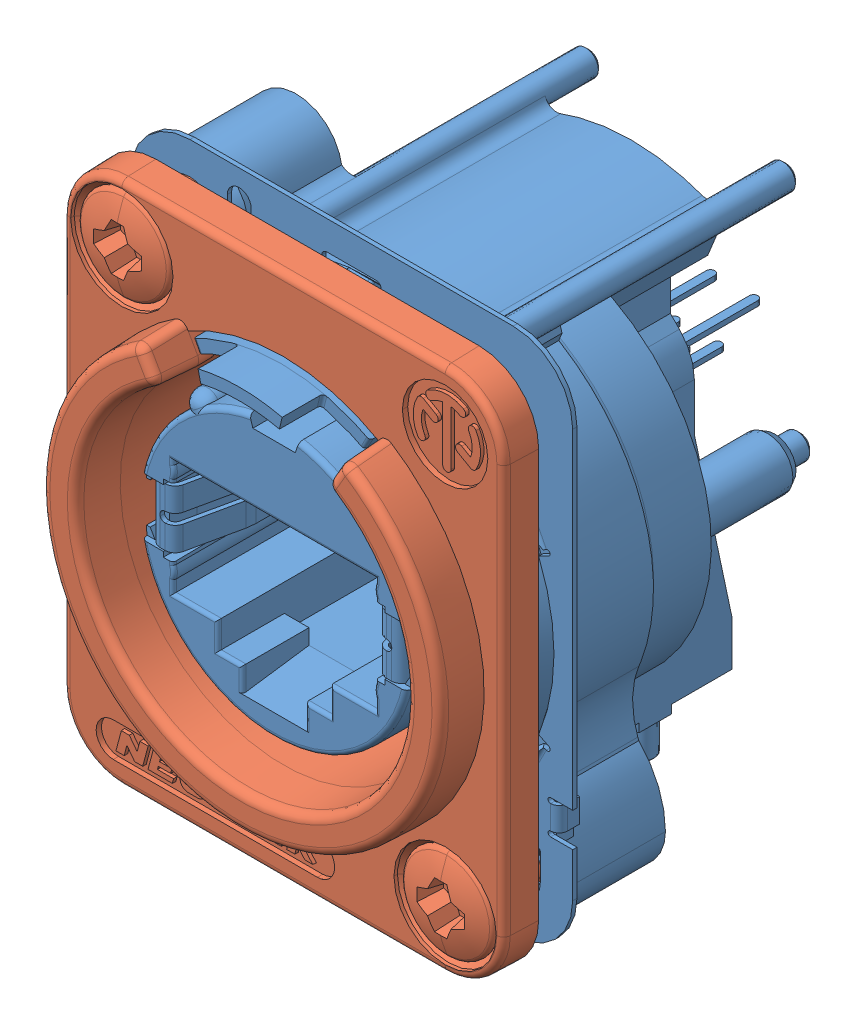
SolidWorks assembly ne8fdh body, configuration Standard. Lengths in mm.
Overall size (26 33.73 26.34).
4 component instances, 3 part files, 3 mates.
Components (placement in the parent):
- ne8fdv.stp-1: ne8fdv.stp [Standard] at origin size (26 32.13 28.88)
  - NE8FDV.stp-1: NE8FDV.stp [Standard] at origin size (26 32.13 28.88)
  - NE8FD.stp-1: NE8FD.stp [Standard] at (0 0 -2.55) size (26 31 14.08) (hidden)
- gnd pin-1: gnd pin [Standard] at (0 0.425 0.0183) size (2.21 8.86 2.48)
Mates (geometry in assembly coordinates):
- Deckungsgleich1: coincident aligned: plane of ne8fdv.stp-1/NE8FDV.stp-1 through (-8.4 -6.1125 -4.675) normal (-1 0 0); plane of gnd pin-1 through (-8.4 -10.55 -9.7875) normal (-1 0 0)
- Deckungsgleich2: coincident aligned: plane of ne8fdv.stp-1/NE8FDV.stp-1 through (0 -10.675 -15.622) normal (0 -1 0); plane of gnd pin-1 through (0 -10.675 -15.9) normal (0 -1 0)
- Deckungsgleich3: coincident aligned: plane of ne8fdv.stp-1/NE8FDV.stp-1 through (-6.6 -11.8238 -16.2) normal (0 0 -1); plane of gnd pin-1 through (0 -10.6003 -16.2) normal (0 0 -1)
